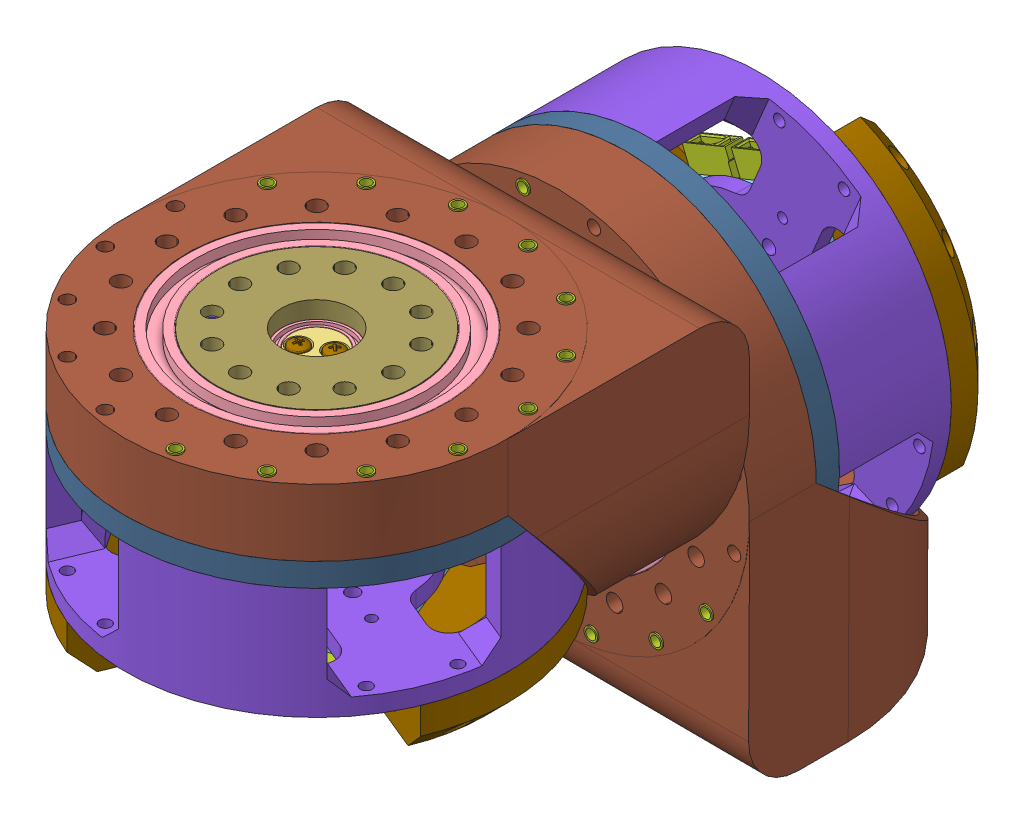
SolidWorks assembly hip, configuration Default. Lengths in mm. (continued)
Components (placement in the parent): (continued)
- Cycloidal_v3-1: Cycloidal_v3 [Default] at (-2.6595 13.4678 32.6634) size (150.25 88 150.25) (continued)
  - foc-motor-controller.step-1: foc-motor-controller.step [Default] at (47.267 33.7573 89.1587) x (-0.382683 0 -0.92388) z (0 -1 0) size (57.23 50 8.13) (continued)
    - R_0603_1608Metric.step-18: R_0603_1608Metric.step [Default] at (-13.3 -20.3875 1.595) x (0 -1 0) z (0 0 1) size (1.6 0.8 0.45)
    - R_0603_1608Metric.step-19: R_0603_1608Metric.step [Default] at (-15.1 -20.3875 1.595) x (0 -1 0) z (0 0 1) size (1.6 0.8 0.45)
    - C_0603_1608Metric.step-17: C_0603_1608Metric.step [Default] at (15.5 -14.4 1.595) x (0 -1 0) z (0 0 1) size (1.6 0.8 0.8)
    - LED_0603_1608Metric.step-1: LED_0603_1608Metric.step [Default] at (-11.5 -23.3875 1.595) x (0 1 0) z (0 0 1) size (1.6 0.8 1.1)
    - C_0805_2012Metric.step-1: C_0805_2012Metric.step [Default] at (19.95 -17 1.595) size (2 1.25 1.25)
    - D_SMB.step-1: D_SMB.step [Default] at (-16.5 11.208 1.595) x (0 -1 0) z (0 0 1) size (5.3 3.55 2.15)
    - C_1206_3216Metric.step-9: C_1206_3216Metric.step [Default] at (-5.3 11 1.595) x (0 1 0) z (0 0 1) size (3.2 1.6 1.6)
    - XT30PW_2_2_-M.G.B.step-2: XT30PW_2_2_-M.G.B.step [Default] at (-20.5 -6.5 1.595) x (0 -1 0) z (-1 0 0) size (15.5 7.1 12.53)
    - C_1206_3216Metric.step-10: C_1206_3216Metric.step [Default] at (1.7 11 1.595) x (0 1 0) z (0 0 1) size (3.2 1.6 1.6)
    - C_1206_3216Metric.step-11: C_1206_3216Metric.step [Default] at (11 11 1.595) x (0 1 0) z (0 0 1) size (3.2 1.6 1.6)
    - C_0603_1608Metric.step-18: C_0603_1608Metric.step [Default] at (-6.3 3.775 1.595) x (0 -1 0) z (0 0 1) size (1.6 0.8 0.8)
    - C_0603_1608Metric.step-19: C_0603_1608Metric.step [Default] at (16.8686 1.7314 1.595) x (0.707107 0.707107 0) z (0 0 1) size (1.6 0.8 0.8)
    - C_0603_1608Metric.step-20: C_0603_1608Metric.step [Default] at (-15.0105 -11.1 1.595) size (1.6 0.8 0.8)
    - C_1206_3216Metric.step-12: C_1206_3216Metric.step [Default] at (-7.7 11 1.595) x (0 1 0) z (0 0 1) size (3.2 1.6 1.6)
    - C_0603_1608Metric.step-21: C_0603_1608Metric.step [Default] at (-18.2 -15.8 1.595) size (1.6 0.8 0.8)
    - C_0603_1608Metric.step-22: C_0603_1608Metric.step [Default] at (-2.1 -11.3 1.595) x (0 -1 0) z (0 0 1) size (1.6 0.8 0.8)
    - C_0603_1608Metric.step-23: C_0603_1608Metric.step [Default] at (-10.8105 -13.4971 1.595) size (1.6 0.8 0.8)
    - C_1206_3216Metric.step-13: C_1206_3216Metric.step [Default] at (4 11 1.595) x (0 1 0) z (0 0 1) size (3.2 1.6 1.6)
    - R_0603_1608Metric.step-20: R_0603_1608Metric.step [Default] at (16 -17.8 1.595) x (0 1 0) z (0 0 1) size (1.6 0.8 0.45)
    - Texas_S-PVSON-N8.step-1: Texas_S-PVSON-N8.step [Default] at (-14.4105 -13.7 1.595) x (-1 0 0) z (0 0 1) size (3 2.98 0.92)
    - C_1206_3216Metric.step-14: C_1206_3216Metric.step [Default] at (21 -2.9 1.595) x (0.707107 -0.707107 0) z (0 0 1) size (3.2 1.6 1.6)
    - C_0603_1608Metric.step-24: C_0603_1608Metric.step [Default] at (-5.9 -16.6 1.595) x (0 1 0) z (0 0 1) size (1.6 0.8 0.8)
    - C_0603_1608Metric.step-25: C_0603_1608Metric.step [Default] at (-3.1 -14.1 1.595) size (1.6 0.8 0.8)
    - R_0603_1608Metric.step-21: R_0603_1608Metric.step [Default] at (7.2 -7.375 1.595) x (0 -1 0) z (0 0 1) size (1.6 0.8 0.45)
    - C_1206_3216Metric.step-15: C_1206_3216Metric.step [Default] at (-0.7 11 1.595) x (0 1 0) z (0 0 1) size (3.2 1.6 1.6)
    - LQFP-64_10x10mm_P0.5mm.step-1: LQFP-64_10x10mm_P0.5mm.step [Default] at (-7 -4.5 1.595) x (-1 0 0) z (0 0 1) size (12 12 1.5)
    - C_0805_2012Metric.step-2: C_0805_2012Metric.step [Default] at (23.35 -17 1.595) x (-1 0 0) z (0 0 1) size (2 1.25 1.25)
    - C_0603_1608Metric.step-26: C_0603_1608Metric.step [Default] at (10.8 -16.8 1.595) x (0 -1 0) z (0 0 1) size (1.6 0.8 0.8)
    - R_0603_1608Metric.step-22: R_0603_1608Metric.step [Default] at (17.5 -17.8 1.595) x (0 -1 0) z (0 0 1) size (1.6 0.8 0.45)
    - C_1206_3216Metric.step-16: C_1206_3216Metric.step [Default] at (20.3 11 1.595) x (0 1 0) z (0 0 1) size (3.2 1.6 1.6)
    - R_0603_1608Metric.step-23: R_0603_1608Metric.step [Default] at (9.2 -16.8 1.595) x (0 -1 0) z (0 0 1) size (1.6 0.8 0.45)
    - C_1206_3216Metric.step-17: C_1206_3216Metric.step [Default] at (-10 11 1.595) x (0 1 0) z (0 0 1) size (3.2 1.6 1.6)
    - R_0603_1608Metric.step-24: R_0603_1608Metric.step [Default] at (17.8 -15.2 1.595) size (1.6 0.8 0.45)
    - C_1206_3216Metric.step-18: C_1206_3216Metric.step [Default] at (19.9 2.6 1.595) x (-0.707107 0.707107 0) z (0 0 1) size (3.2 1.6 1.6)
    - C_0603_1608Metric.step-27: C_0603_1608Metric.step [Default] at (13.4 -7.375 1.595) x (0 -1 0) z (0 0 1) size (1.6 0.8 0.8)
    - R_0603_1608Metric.step-25: R_0603_1608Metric.step [Default] at (8.7 -7.375 1.595) x (0 -1 0) z (0 0 1) size (1.6 0.8 0.45)
    - PQFN-8-EP_6x5mm_P1.27mm_Generic.step-1: PQFN-8-EP_6x5mm_P1.27mm_Generic.step [Default] at (4.9 14.4 -0.085) x (0 1 0) z (0 0 -1) size (6.15 5.15 1.09)
    - C_0805_2012Metric.step-3: C_0805_2012Metric.step [Default] at (-3 8.9 -0.085) x (0 1 0) z (0 0 -1) size (2 1.25 1.25)
    - C_0603_1608Metric.step-28: C_0603_1608Metric.step [Default] at (1.5 -4.3 -0.085) x (0 1 0) z (0 0 -1) size (1.6 0.8 0.8)
    - R_2512_6332Metric.step-1: R_2512_6332Metric.step [Default] at (2.1 8.6 -0.085) x (-1 0 0) z (0 0 -1) size (6.3 3.2 0.6)
    - C_0805_2012Metric.step-4: C_0805_2012Metric.step [Default] at (18.8 8.9 -0.085) x (0 1 0) z (0 0 -1) size (2 1.25 1.25)
    - C_0805_2012Metric.step-5: C_0805_2012Metric.step [Default] at (-5.2 8.901 -0.085) x (0 1 0) z (0 0 -1) size (2 1.25 1.25)
    - PQFN-8-EP_6x5mm_P1.27mm_Generic.step-2: PQFN-8-EP_6x5mm_P1.27mm_Generic.step [Default] at (16.9 14.6 -0.085) x (0 -1 0) z (0 0 -1) size (6.15 5.15 1.09)
    - PQFN-8-EP_6x5mm_P1.27mm_Generic.step-3: PQFN-8-EP_6x5mm_P1.27mm_Generic.step [Default] at (-1.1 14.6 -0.085) x (0 -1 0) z (0 0 -1) size (6.15 5.15 1.09)
    - R_0603_1608Metric.step-26: R_0603_1608Metric.step [Default] at (8.2 8.8 -0.085) x (0 1 0) z (0 0 -1) size (1.6 0.8 0.45)
    - R_2512_6332Metric.step-2: R_2512_6332Metric.step [Default] at (-10.3 8.601 -0.085) x (1 0 0) z (0 0 -1) size (6.3 3.2 0.6)
    - TSSOP-16_4.4x5mm_P0.65mm.step-1: TSSOP-16_4.4x5mm_P0.65mm.step [Default] at (0 0 -0.085) x (-1 0 0) z (0 0 -1) size (6.4 5 1.1)
    - C_0603_1608Metric.step-29: C_0603_1608Metric.step [Default] at (0 -4.25 -0.085) x (0 1 0) z (0 0 -1) size (1.6 0.8 0.8)
    - PQFN-8-EP_6x5mm_P1.27mm_Generic.step-4: PQFN-8-EP_6x5mm_P1.27mm_Generic.step [Default] at (10.9 14.4 -0.085) x (0 1 0) z (0 0 -1) size (6.15 5.15 1.09)
    - R_2512_6332Metric.step-3: R_2512_6332Metric.step [Default] at (13.7 8.6 -0.085) x (1 0 0) z (0 0 -1) size (6.3 3.2 0.6)
    - PQFN-8-EP_6x5mm_P1.27mm_Generic.step-5: PQFN-8-EP_6x5mm_P1.27mm_Generic.step [Default] at (-13.1 14.401 -0.085) x (0 1 0) z (0 0 -1) size (6.15 5.15 1.09)
    - C_0603_1608Metric.step-30: C_0603_1608Metric.step [Default] at (-1.5 -4.3 -0.085) x (0 -1 0) z (0 0 -1) size (1.6 0.8 0.8)
    - PQFN-8-EP_6x5mm_P1.27mm_Generic.step-6: PQFN-8-EP_6x5mm_P1.27mm_Generic.step [Default] at (-7.1 14.601 -0.085) x (0 -1 0) z (0 0 -1) size (6.15 5.15 1.09)
    - foc-motor-controller_PCB.step-1: foc-motor-controller_PCB.step [Default] at origin size (50 50 1.51)
  - hex nut style 1 gradeab_iso-1: hex nut style 1 gradeab_iso [ISO - 4032 - M3 - W - N] at (35.6313 33.7573 117.2498) x (1 0 0) z (0 -1 0) size (5.5 6.35 2.4)
  - Cycloidal_Discs_8308-1: Cycloidal_Discs_8308 [Default] at (6.9481 42.227 30.6143) x (0.999764 0 -0.021738) z (0.021738 0 0.999764) size (79.25 5 79.73)
    - Cycloidal_Discs-1: Cycloidal_Discs [Default] at (38.3081 39.5303 58.0959) size (79.25 5 79.73)
    - radial ball bearing_68_iso-1: radial ball bearing_68_iso [ISO 15 RBB - 274 - 14,SI,NC,14_68] at (18.3896 43.2803 46.5959) x (0 1 0) z (0 0 1) size (2.5 7 7)
    - radial ball bearing_68_iso-2: radial ball bearing_68_iso [ISO 15 RBB - 274 - 14,SI,NC,14_68] at (38.3081 43.2803 81.0959) x (0 1 0) z (0 0 1) size (2.5 7 7)
    - radial ball bearing_68_iso-3: radial ball bearing_68_iso [ISO 15 RBB - 274 - 14,SI,NC,14_68] at (18.3896 43.2803 69.5959) x (0 1 0) z (0 0 1) size (2.5 7 7)
    - radial ball bearing_68_iso-4: radial ball bearing_68_iso [ISO 15 RBB - 274 - 14,SI,NC,14_68] at (38.3081 43.2803 35.0959) x (0 1 0) z (0 0 1) size (2.5 7 7)
    - radial ball bearing_68_iso-5: radial ball bearing_68_iso [ISO 15 RBB - 274 - 14,SI,NC,14_68] at (58.2267 43.2803 69.5959) x (0 1 0) z (0 0 1) size (2.5 7 7)
    - radial ball bearing_68_iso-6: radial ball bearing_68_iso [ISO 15 RBB - 274 - 14,SI,NC,14_68] at (58.2267 43.2803 46.5959) x (0 1 0) z (0 0 1) size (2.5 7 7)
  - Cycloidal_Discs_8308-2: Cycloidal_Discs_8308 [Default] at (85.7348 37.227 31.9683) x (0.403317 0 0.91506) z (-0.91506 0 0.403317) size (79.25 5 79.73)
    - Cycloidal_Discs-1: Cycloidal_Discs [Default] at (38.3081 39.5303 58.0959) size (79.25 5 79.73)
    - radial ball bearing_68_iso-1: radial ball bearing_68_iso [ISO 15 RBB - 274 - 14,SI,NC,14_68] at (18.3896 43.2803 46.5959) x (0 1 0) z (0 0 1) size (2.5 7 7)
    - radial ball bearing_68_iso-2: radial ball bearing_68_iso [ISO 15 RBB - 274 - 14,SI,NC,14_68] at (38.3081 43.2803 81.0959) x (0 1 0) z (0 0 1) size (2.5 7 7)
    - radial ball bearing_68_iso-3: radial ball bearing_68_iso [ISO 15 RBB - 274 - 14,SI,NC,14_68] at (18.3896 43.2803 69.5959) x (0 1 0) z (0 0 1) size (2.5 7 7)
    - radial ball bearing_68_iso-4: radial ball bearing_68_iso [ISO 15 RBB - 274 - 14,SI,NC,14_68] at (38.3081 43.2803 35.0959) x (0 1 0) z (0 0 1) size (2.5 7 7)
    - radial ball bearing_68_iso-5: radial ball bearing_68_iso [ISO 15 RBB - 274 - 14,SI,NC,14_68] at (58.2267 43.2803 69.5959) x (0 1 0) z (0 0 1) size (2.5 7 7)
    - radial ball bearing_68_iso-6: radial ball bearing_68_iso [ISO 15 RBB - 274 - 14,SI,NC,14_68] at (58.2267 43.2803 46.5959) x (0 1 0) z (0 0 1) size (2.5 7 7)
  - m6-1: m6 [Default] at (27.3484 93.9895 100.6587) x (-0.80367 0 -0.595076) z (-0.595076 0 0.80367) size (6 16 6)
  - Motor_Cover_v2-2: Motor_Cover_v2 [Default] at (47.267 36.1573 89.1587) x (-0.92388 0 -0.382683) z (0.382683 0 -0.92388) size (115 33.6 115)
  - driver_cover-1: driver_cover [Default] at (47.267 36.1573 89.1587) x (-0.384295 0 -0.92321) z (-0.92321 0 0.384295) size (81.32 15 115)
  - Base_plate_2-1: Base_plate_2 [Default] at (47.267 69.7573 89.1587) size (115 7 115)
  - Cover_new-1: Cover_new [Default] at (47.267 86.8173 89.1587) size (115 87.56 130)
  - Output_Shaft-1: Output_Shaft [Default] at (47.267 86.8173 89.1587) size (60 10 60)
- Cycloidal_v3-2: Cycloidal_v3 [Default] at (91.3873 -36.6902 -47.4953) x (-0.999985 0.005457 0) z (0.005457 0.999985 0) size (150.25 88 150.25)
  - motor-X83008S.stp-1: motor-X83008S.stp [Default] at (85.5027 89.8915 67.8666) x (-0.706334 0 0.707879) z (0 -1 0) size (114.7 114.7 37.62) (hidden)
    - base.stp-1: base.stp [Default] at (42.0794 12.0269 46.7342) size (91.6 91.6 15.61)
    - stator.stp-1: stator.stp [Default] at (42.0794 12.0269 33.1342) x (0.08493 -0.996387 0) z (0 0 1) size (83 83 8)
    - coil.stp-1: coil.stp [Default] at (39.5332 41.8984 37.1342) x (0.996387 0.08493 0) z (-0.08493 0.996387 0) size (4.4 10.2 10.5)
    - coil.stp-2: coil.stp [Default] at (34.3848 41.0025 37.1342) x (0.966502 0.256661 0) z (-0.256661 0.966502 0) size (4.4 10.2 10.5)
    - coil.stp-3: coil.stp [Default] at (29.4701 39.2261 37.1342) x (0.90725 0.420593 0) z (-0.420593 0.90725 0) size (4.4 10.2 10.5)
    - coil.stp-4: coil.stp [Default] at (24.9386 36.6233 37.1342) x (0.820431 0.571745 0) z (-0.571745 0.820431 0) size (4.4 10.2 10.5)
    - coil.stp-5: coil.stp [Default] at (20.9279 33.2732 37.1342) x (0.708685 0.705525 0) z (-0.705525 0.708685 0) size (4.4 10.2 10.5)
    - coil.stp-6: coil.stp [Default] at (17.5599 29.2775 37.1342) x (0.575405 0.817869 0) z (-0.817869 0.575405 0) size (4.4 10.2 10.5)
    - coil.stp-7: coil.stp [Default] at (14.9368 24.7576 37.1342) x (0.424642 0.905361 0) z (-0.905361 0.424642 0) size (4.4 10.2 10.5)
    - coil.stp-8: coil.stp [Default] at (13.1385 19.8509 37.1342) x (0.260976 0.965345 0) z (-0.965345 0.260976 0) size (4.4 10.2 10.5)
    - coil.stp-9: coil.stp [Default] at (12.2196 14.7066 37.1342) x (0.089381 0.995998 0) z (-0.995998 0.089381 0) size (4.4 10.2 10.5)
    - coil.stp-10: coil.stp [Default] at (12.2079 9.4807 37.1342) x (-0.08493 0.996387 0) z (-0.996387 -0.08493 0) size (4.4 10.2 10.5)
    - coil.stp-11: coil.stp [Default] at (13.1039 4.3323 37.1342) x (-0.256661 0.966502 0) z (-0.966502 -0.256661 0) size (4.4 10.2 10.5)
    - coil.stp-12: coil.stp [Default] at (14.8802 -0.5824 37.1342) x (-0.420593 0.90725 0) z (-0.90725 -0.420593 0) size (4.4 10.2 10.5)
    - coil.stp-13: coil.stp [Default] at (17.483 -5.1139 37.1342) x (-0.571745 0.820431 0) z (-0.820431 -0.571745 0) size (4.4 10.2 10.5)
    - coil.stp-14: coil.stp [Default] at (20.8332 -9.1246 37.1342) x (-0.705525 0.708685 0) z (-0.708685 -0.705525 0) size (4.4 10.2 10.5)
    - coil.stp-15: coil.stp [Default] at (24.8289 -12.4926 37.1342) x (-0.817869 0.575405 0) z (-0.575405 -0.817869 0) size (4.4 10.2 10.5)
    - coil.stp-16: coil.stp [Default] at (29.3487 -15.1157 37.1342) x (-0.905361 0.424642 0) z (-0.424642 -0.905361 0) size (4.4 10.2 10.5)
    - coil.stp-17: coil.stp [Default] at (34.2554 -16.914 37.1342) x (-0.965345 0.260976 0) z (-0.260976 -0.965345 0) size (4.4 10.2 10.5)
    - coil.stp-18: coil.stp [Default] at (39.3998 -17.8329 37.1342) x (-0.995998 0.089381 0) z (-0.089381 -0.995998 0) size (4.4 10.2 10.5)
    - coil.stp-19: coil.stp [Default] at (44.6256 -17.8446 37.1342) x (-0.996387 -0.08493 0) z (0.08493 -0.996387 0) size (4.4 10.2 10.5)
    - coil.stp-20: coil.stp [Default] at (49.7741 -16.9486 37.1342) x (-0.966502 -0.256661 0) z (0.256661 -0.966502 0) size (4.4 10.2 10.5)
    - coil.stp-21: coil.stp [Default] at (54.6887 -15.1723 37.1342) x (-0.90725 -0.420593 0) z (0.420593 -0.90725 0) size (4.4 10.2 10.5)
    - coil.stp-22: coil.stp [Default] at (59.2202 -12.5695 37.1342) x (-0.820431 -0.571745 0) z (0.571745 -0.820431 0) size (4.4 10.2 10.5)
    - coil.stp-23: coil.stp [Default] at (63.2309 -9.2193 37.1342) x (-0.708685 -0.705525 0) z (0.705525 -0.708685 0) size (4.4 10.2 10.5)
    - coil.stp-24: coil.stp [Default] at (66.599 -5.2236 37.1342) x (-0.575405 -0.817869 0) z (0.817869 -0.575405 0) size (4.4 10.2 10.5)
    - coil.stp-25: coil.stp [Default] at (69.222 -0.7038 37.1342) x (-0.424642 -0.905361 0) z (0.905361 -0.424642 0) size (4.4 10.2 10.5)
    - coil.stp-26: coil.stp [Default] at (71.0203 4.2029 37.1342) x (-0.260976 -0.965345 0) z (0.965345 -0.260976 0) size (4.4 10.2 10.5)
    - coil.stp-27: coil.stp [Default] at (71.9392 9.3473 37.1342) x (-0.089381 -0.995998 0) z (0.995998 -0.089381 0) size (4.4 10.2 10.5)
    - coil.stp-28: coil.stp [Default] at (71.9509 14.5731 37.1342) x (0.08493 -0.996387 0) z (0.996387 0.08493 0) size (4.4 10.2 10.5)
    - coil.stp-29: coil.stp [Default] at (71.055 19.7216 37.1342) x (0.256661 -0.966502 0) z (0.966502 0.256661 0) size (4.4 10.2 10.5)
    - coil.stp-30: coil.stp [Default] at (69.2786 24.6362 37.1342) x (0.420593 -0.90725 0) z (0.90725 0.420593 0) size (4.4 10.2 10.5)
    - coil.stp-31: coil.stp [Default] at (66.6758 29.1677 37.1342) x (0.571745 -0.820431 0) z (0.820431 0.571745 0) size (4.4 10.2 10.5)
    - coil.stp-32: coil.stp [Default] at (63.3257 33.1785 37.1342) x (0.705525 -0.708685 0) z (0.708685 0.705525 0) size (4.4 10.2 10.5)
    - coil.stp-33: coil.stp [Default] at (59.33 36.5465 37.1342) x (0.817869 -0.575405 0) z (0.575405 0.817869 0) size (4.4 10.2 10.5)
    - coil.stp-34: coil.stp [Default] at (54.8101 39.1695 37.1342) x (0.905361 -0.424642 0) z (0.424642 0.905361 0) size (4.4 10.2 10.5)
    - coil.stp-35: coil.stp [Default] at (49.9034 40.9678 37.1342) x (0.965345 -0.260976 0) z (0.260976 0.965345 0) size (4.4 10.2 10.5)
    - coil.stp-36: coil.stp [Default] at (44.759 41.8868 37.1342) x (0.995998 -0.089381 0) z (0.089381 0.995998 0) size (4.4 10.2 10.5)
    - rotor.stp-1: rotor.stp [Default] at (42.0794 12.0269 42.1342) x (-0.293442 0.955977 0) z (0 0 -1) size (91.8 91.8 12)
    - outrunner.stp-1: outrunner.stp [Default] at (42.0794 12.0269 30.1342) x (-0.254711 0.967017 0) z (-0.967017 -0.254711 0) size (91.8 17.01 91.8)
    - screw-mount.stp-1: screw-mount.stp [Default] at (38.1314 27.0157 27.1342) x (1 0 0) z (0 0 -1) size (7 7 6.5)
    - screw-mount.stp-2: screw-mount.stp [Default] at (27.0906 8.0789 27.1342) x (1 0 0) z (0 0 -1) size (7 7 6.5)
    - screw-mount.stp-3: screw-mount.stp [Default] at (57.0682 15.9749 27.1342) x (1 0 0) z (0 0 -1) size (7 7 6.5)
    - screw-mount.stp-4: screw-mount.stp [Default] at (46.0274 -2.9618 27.1342) x (1 0 0) z (0 0 -1) size (7 7 6.5)
    - 6702ZZ-bearing-15x21x4.stp-1: 6702ZZ-bearing-15x21x4.stp [Default] at (42.0794 12.0269 43.7342) x (1 0 0) z (0 -1 0) size (21 4 21)
    - 6702ZZ-bearing-15x21x4.stp-2: 6702ZZ-bearing-15x21x4.stp [Default] at (42.0794 12.0269 35.1342) x (1 0 0) z (0 1 0) size (21 4 21)
    - shaft.stp-1: shaft.stp [Default] at (42.0794 12.0269 20.1342) size (16 16 31.6)
    - fix-screw.stp-1: fix-screw.stp [Default] at (42.0794 12.0269 51.7342) x (1 0 0) z (0 0 -1) size (19.67 18.96 12.02)
  - Base_Plate-1: Base_Plate [Default] at (47.267 69.7573 89.1587) x (0.863342 0 -0.50462) z (0.50462 0 0.863342) size (40 7 40)
  - Eccentric_Shaft-1: Eccentric_Shaft [Default] at (38.9525 70.4165 102.8564) x (-0.50462 0 -0.863342) z (0.863342 0 -0.50462) size (20 15 17)
    - Eccentric_Shaft_bot-1: Eccentric_Shaft_bot [Default] at (7.6302 6.3409 14.0904) size (17 5 17)
    - Eccentric_Shaft_bot-2: Eccentric_Shaft_bot [Default] at (7.6302 11.3409 14.0904) x (-1 0 0) z (0 0 -1) size (17 5 17)
    - Eccentric_Shaft_top-1: Eccentric_Shaft_top [Default] at (7.6302 16.3409 14.0904) x (-1 0 0) z (0 0 -1) size (17 5 17)
  - radial ball bearing_68_iso-39: radial ball bearing_68_iso [ISO 15 RBB - 1860 - 32,SI,NC,32_68] at (47.267 91.8173 89.1587) x (0 1 0) z (0.105786 0 0.994389) size (10 78 78)
  - radial ball bearing_68_iso-40: radial ball bearing_68_iso [ISO 15 RBB - 1840 - 32,SI,NC,32_68] at (47.267 73.2573 89.1587) x (0 1 0) z (-0.019534 0 0.999809) size (7 52 52)
  - m13_bearing-31: m13_bearing [Default] at (-10.7414 95.4081 67.0593) x (0.227678 0 0.973736) z (0.973736 0 -0.227678) size (13 16 13)
    - m6-1: m6 [Default] at (8.4921 2.5508 14.8914) size (6 16 6)
    - radial ball bearing_68_iso-1: radial ball bearing_68_iso [ISO 15 RBB - 286 - 10,SI,NC,10_68] at (8.4921 16.0508 14.8914) x (0 1 0) z (0 0 1) size (5 13 13)
    - radial ball bearing_68_iso-2: radial ball bearing_68_iso [ISO 15 RBB - 286 - 10,SI,NC,10_68] at (8.4921 11.0508 14.8914) x (0 1 0) z (0 0 1) size (5 13 13)
  - m13_bearing-32: m13_bearing [Default] at (-14.1668 95.4081 84.2801) x (0.227678 0 0.973736) z (0.973736 0 -0.227678) size (13 16 13)
    - m6-1: m6 [Default] at (8.4921 2.5508 14.8914) size (6 16 6)
    - radial ball bearing_68_iso-1: radial ball bearing_68_iso [ISO 15 RBB - 286 - 10,SI,NC,10_68] at (8.4921 16.0508 14.8914) x (0 1 0) z (0 0 1) size (5 13 13)
    - radial ball bearing_68_iso-2: radial ball bearing_68_iso [ISO 15 RBB - 286 - 10,SI,NC,10_68] at (8.4921 11.0508 14.8914) x (0 1 0) z (0 0 1) size (5 13 13)
  - m13_bearing-34: m13_bearing [Default] at (13.6125 95.5581 125.8547) x (0.227678 0 0.973736) z (0.973736 0 -0.227678) size (13 16 13)
    - m6-1: m6 [Default] at (8.4921 2.5508 14.8914) size (6 16 6)
    - radial ball bearing_68_iso-1: radial ball bearing_68_iso [ISO 15 RBB - 286 - 10,SI,NC,10_68] at (8.4921 16.0508 14.8914) x (0 1 0) z (0 0 1) size (5 13 13)
    - radial ball bearing_68_iso-2: radial ball bearing_68_iso [ISO 15 RBB - 286 - 10,SI,NC,10_68] at (8.4921 11.0508 14.8914) x (0 1 0) z (0 0 1) size (5 13 13)
  - m13_bearing-35: m13_bearing [Default] at (-0.9866 95.4081 116.0999) x (0.227678 0 0.973736) z (0.973736 0 -0.227678) size (13 16 13)
    - m6-1: m6 [Default] at (8.4921 2.5508 14.8914) size (6 16 6)
    - radial ball bearing_68_iso-1: radial ball bearing_68_iso [ISO 15 RBB - 286 - 10,SI,NC,10_68] at (8.4921 16.0508 14.8914) x (0 1 0) z (0 0 1) size (5 13 13)
    - radial ball bearing_68_iso-2: radial ball bearing_68_iso [ISO 15 RBB - 286 - 10,SI,NC,10_68] at (8.4921 11.0508 14.8914) x (0 1 0) z (0 0 1) size (5 13 13)
  - m13_bearing-36: m13_bearing [Default] at (-10.7414 95.5581 101.5009) x (0.227678 0 0.973736) z (0.973736 0 -0.227678) size (13 16 13)
    - m6-1: m6 [Default] at (8.4921 2.5508 14.8914) size (6 16 6)
    - radial ball bearing_68_iso-1: radial ball bearing_68_iso [ISO 15 RBB - 286 - 10,SI,NC,10_68] at (8.4921 16.0508 14.8914) x (0 1 0) z (0 0 1) size (5 13 13)
    - radial ball bearing_68_iso-2: radial ball bearing_68_iso [ISO 15 RBB - 286 - 10,SI,NC,10_68] at (8.4921 11.0508 14.8914) x (0 1 0) z (0 0 1) size (5 13 13)
  - m13_bearing-1: m13_bearing [Default] at (-0.8801 95.4081 62.5627) x (0.736525 0 0.676411) z (0.676411 0 -0.736525) size (13 16 13)
    - m6-1: m6 [Default] at (8.4921 2.5508 14.8914) size (6 16 6)
    - radial ball bearing_68_iso-1: radial ball bearing_68_iso [ISO 15 RBB - 286 - 10,SI,NC,10_68] at (8.4921 16.0508 14.8914) x (0 1 0) z (0 0 1) size (5 13 13)
    - radial ball bearing_68_iso-2: radial ball bearing_68_iso [ISO 15 RBB - 286 - 10,SI,NC,10_68] at (8.4921 11.0508 14.8914) x (0 1 0) z (0 0 1) size (5 13 13)
  - m13_bearing-2: m13_bearing [Default] at (48.6831 95.4081 124.0939) x (0.120271 0 0.992741) z (0.992741 0 -0.120271) size (13 16 13)
    - m6-1: m6 [Default] at (8.4921 2.5508 14.8914) size (6 16 6)
    - radial ball bearing_68_iso-1: radial ball bearing_68_iso [ISO 15 RBB - 286 - 10,SI,NC,10_68] at (8.4921 16.0508 14.8914) x (0 1 0) z (0 0 1) size (5 13 13)
    - radial ball bearing_68_iso-2: radial ball bearing_68_iso [ISO 15 RBB - 286 - 10,SI,NC,10_68] at (8.4921 11.0508 14.8914) x (0 1 0) z (0 0 1) size (5 13 13)
  - m13_bearing-3: m13_bearing [Default] at (32.7832 95.4081 34.9886) x (-0.046141 0 0.998935) z (0.998935 0 0.046141) size (13 16 13)
    - m6-1: m6 [Default] at (8.4921 2.5508 14.8914) size (6 16 6)
    - radial ball bearing_68_iso-1: radial ball bearing_68_iso [ISO 15 RBB - 286 - 10,SI,NC,10_68] at (8.4921 16.0508 14.8914) x (0 1 0) z (0 0 1) size (5 13 13)
    - radial ball bearing_68_iso-2: radial ball bearing_68_iso [ISO 15 RBB - 286 - 10,SI,NC,10_68] at (8.4921 11.0508 14.8914) x (0 1 0) z (0 0 1) size (5 13 13)
  - m13_bearing-4: m13_bearing [Default] at (77.6928 95.3081 80.133) x (-0.036208 0 0.999344) z (0.999344 0 0.036208) size (13 16 13)
    - m6-1: m6 [Default] at (8.4921 2.5508 14.8914) size (6 16 6)
    - radial ball bearing_68_iso-1: radial ball bearing_68_iso [ISO 15 RBB - 286 - 10,SI,NC,10_68] at (8.4921 16.0508 14.8914) x (0 1 0) z (0 0 1) size (5 13 13)
    - radial ball bearing_68_iso-2: radial ball bearing_68_iso [ISO 15 RBB - 286 - 10,SI,NC,10_68] at (8.4921 11.0508 14.8914) x (0 1 0) z (0 0 1) size (5 13 13)
  - m13_bearing-5: m13_bearing [Default] at (73.474 95.4081 98.7828) x (0.059133 0 0.99825) z (0.99825 0 -0.059133) size (13 16 13)
    - m6-1: m6 [Default] at (8.4921 2.5508 14.8914) size (6 16 6)
    - radial ball bearing_68_iso-1: radial ball bearing_68_iso [ISO 15 RBB - 286 - 10,SI,NC,10_68] at (8.4921 16.0508 14.8914) x (0 1 0) z (0 0 1) size (5 13 13)
    - radial ball bearing_68_iso-2: radial ball bearing_68_iso [ISO 15 RBB - 286 - 10,SI,NC,10_68] at (8.4921 11.0508 14.8914) x (0 1 0) z (0 0 1) size (5 13 13)
  - m13_bearing-6: m13_bearing [Default] at (12.9248 95.4081 46.7315) x (0.451561 0 0.89224) z (0.89224 0 -0.451561) size (13 16 13)
    - m6-1: m6 [Default] at (8.4921 2.5508 14.8914) size (6 16 6)
    - radial ball bearing_68_iso-1: radial ball bearing_68_iso [ISO 15 RBB - 286 - 10,SI,NC,10_68] at (8.4921 16.0508 14.8914) x (0 1 0) z (0 0 1) size (5 13 13)
    - radial ball bearing_68_iso-2: radial ball bearing_68_iso [ISO 15 RBB - 286 - 10,SI,NC,10_68] at (8.4921 11.0508 14.8914) x (0 1 0) z (0 0 1) size (5 13 13)
  - m13_bearing-7: m13_bearing [Default] at (56.6452 95.4081 32.3406) x (-0.545813 0 0.837907) z (0.837907 0 0.545813) size (13 16 13)
    - m6-1: m6 [Default] at (8.4921 2.5508 14.8914) size (6 16 6)
    - radial ball bearing_68_iso-1: radial ball bearing_68_iso [ISO 15 RBB - 286 - 10,SI,NC,10_68] at (8.4921 16.0508 14.8914) x (0 1 0) z (0 0 1) size (5 13 13)
    - radial ball bearing_68_iso-2: radial ball bearing_68_iso [ISO 15 RBB - 286 - 10,SI,NC,10_68] at (8.4921 11.0508 14.8914) x (0 1 0) z (0 0 1) size (5 13 13)
  - m13_bearing-8: m13_bearing [Default] at (63.0373 95.4081 51.3153) x (0.158553 0 0.98735) z (0.98735 0 -0.158553) size (13 16 13)
    - m6-1: m6 [Default] at (8.4921 2.5508 14.8914) size (6 16 6)
    - radial ball bearing_68_iso-1: radial ball bearing_68_iso [ISO 15 RBB - 286 - 10,SI,NC,10_68] at (8.4921 16.0508 14.8914) x (0 1 0) z (0 0 1) size (5 13 13)
    - radial ball bearing_68_iso-2: radial ball bearing_68_iso [ISO 15 RBB - 286 - 10,SI,NC,10_68] at (8.4921 11.0508 14.8914) x (0 1 0) z (0 0 1) size (5 13 13)
  - m13_bearing-9: m13_bearing [Default] at (83.8577 95.4081 55.5358) x (-0.687134 0 0.72653) z (0.72653 0 0.687134) size (13 16 13)
    - m6-1: m6 [Default] at (8.4921 2.5508 14.8914) size (6 16 6)
    - radial ball bearing_68_iso-1: radial ball bearing_68_iso [ISO 15 RBB - 286 - 10,SI,NC,10_68] at (8.4921 16.0508 14.8914) x (0 1 0) z (0 0 1) size (5 13 13)
    - radial ball bearing_68_iso-2: radial ball bearing_68_iso [ISO 15 RBB - 286 - 10,SI,NC,10_68] at (8.4921 11.0508 14.8914) x (0 1 0) z (0 0 1) size (5 13 13)
  - m13_bearing-11: m13_bearing [Default] at (30.1977 95.4081 135.7424) x (0.57351 0 0.819198) z (0.819198 0 -0.57351) size (13 16 13)
    - m6-1: m6 [Default] at (8.4921 2.5508 14.8914) size (6 16 6)
    - radial ball bearing_68_iso-1: radial ball bearing_68_iso [ISO 15 RBB - 286 - 10,SI,NC,10_68] at (8.4921 16.0508 14.8914) x (0 1 0) z (0 0 1) size (5 13 13)
    - radial ball bearing_68_iso-2: radial ball bearing_68_iso [ISO 15 RBB - 286 - 10,SI,NC,10_68] at (8.4921 11.0508 14.8914) x (0 1 0) z (0 0 1) size (5 13 13)
  - m13_bearing-12: m13_bearing [Default] at (62.8861 95.4081 115.3744) x (0.184178 0 0.982893) z (0.982893 0 -0.184178) size (13 16 13)
    - m6-1: m6 [Default] at (8.4921 2.5508 14.8914) size (6 16 6)
    - radial ball bearing_68_iso-1: radial ball bearing_68_iso [ISO 15 RBB - 286 - 10,SI,NC,10_68] at (8.4921 16.0508 14.8914) x (0 1 0) z (0 0 1) size (5 13 13)
    - radial ball bearing_68_iso-2: radial ball bearing_68_iso [ISO 15 RBB - 286 - 10,SI,NC,10_68] at (8.4921 11.0508 14.8914) x (0 1 0) z (0 0 1) size (5 13 13)
  - socket button head screw_iso-2: socket button head screw_iso [ISO 7380 - M4 x 12 - 12N] at (47.267 67.4573 134.1587) x (0 1 0) z (-0.724148 0 0.689645) size (14.2 7.6 7.6)
  - socket button head screw_iso-3: socket button head screw_iso [ISO 7380 - M4 x 12 - 12N] at (15.4472 67.4573 57.3389) x (0 1 0) z (-0.724148 0 0.689645) size (14.2 7.6 7.6)
  - socket button head screw_iso-4: socket button head screw_iso [ISO 7380 - M4 x 12 - 12N] at (30.0462 67.4573 47.5841) x (0 1 0) z (-0.724148 0 0.689645) size (14.2 7.6 7.6)
  - socket button head screw_iso-5: socket button head screw_iso [ISO 7380 - M4 x 12 - 12N] at (47.267 67.4573 44.1587) x (0 1 0) z (-0.724148 0 0.689645) size (14.2 7.6 7.6)
  - socket button head screw_iso-6: socket button head screw_iso [ISO 7380 - M4 x 12 - 12N] at (64.4877 67.4573 47.5841) x (0 1 0) z (-0.724148 0 0.689645) size (14.2 7.6 7.6)
  - socket button head screw_iso-8: socket button head screw_iso [ISO 7380 - M4 x 12 - 12N] at (88.8416 67.4573 71.9379) x (0 1 0) z (-0.724148 0 0.689645) size (14.2 7.6 7.6)
  - socket button head screw_iso-9: socket button head screw_iso [ISO 7380 - M4 x 12 - 12N] at (92.267 67.4573 89.1587) x (0 1 0) z (-0.724148 0 0.689645) size (14.2 7.6 7.6)
  - socket button head screw_iso-10: socket button head screw_iso [ISO 7380 - M4 x 12 - 12N] at (88.8416 67.4573 106.3794) x (0 1 0) z (-0.724148 0 0.689645) size (14.2 7.6 7.6)
  - socket button head screw_iso-11: socket button head screw_iso [ISO 7380 - M4 x 12 - 12N] at (79.0868 67.4573 120.9785) x (0 1 0) z (-0.724148 0 0.689645) size (14.2 7.6 7.6)
  - M3x4x4.2_brass_insert-2: M3x4x4.2_brass_insert [Default] at (2.3676 97.2573 59.1579) x (-0.680278 0 -0.732954) z (-0.732954 0 0.680278) size (4 4 4)
  - M3x4x4.2_brass_insert-3: M3x4x4.2_brass_insert [Default] at (17.2662 97.2573 44.2593) x (-0.509546 0 -0.860444) z (-0.860444 0 0.509546) size (4 4 4)
  - M3x4x4.2_brass_insert-6: M3x4x4.2_brass_insert [Default] at (77.2678 97.2573 44.2593) x (-0.680278 0 -0.732954) z (-0.732954 0 0.680278) size (4 4 4)
  - M3x4x4.2_brass_insert-8: M3x4x4.2_brass_insert [Default] at (100.2294 93.2573 78.6238) x (-0.970393 0 0.241533) z (-0.241533 0 -0.970393) size (4 4 4)
  - M3x4x4.2_brass_insert-14: M3x4x4.2_brass_insert [Default] at (36.7321 97.2573 36.1963) x (0.509546 0 0.860444) z (0.860444 0 -0.509546) size (4 4 4)
  - M3x4x4.2_brass_insert-15: M3x4x4.2_brass_insert [Default] at (57.8019 93.2573 36.1963) x (0.897191 0 -0.441644) z (0.441644 0 0.897191) size (4 4 4)
  - M3x4x4.2_brass_insert-16: M3x4x4.2_brass_insert [Default] at (92.1663 97.2573 59.1579) x (-0.680278 0 -0.732954) z (-0.732954 0 0.680278) size (4 4 4)
  - M3x4x4.2_brass_insert-17: M3x4x4.2_brass_insert [Default] at (100.2294 97.2573 99.6935) x (0.680278 0 0.732954) z (0.732954 0 -0.680278) size (4 4 4)
  - M3x4x4.2_brass_insert-19: M3x4x4.2_brass_insert [Default] at (92.1663 97.2573 119.1595) x (0.680278 0 0.732954) z (0.732954 0 -0.680278) size (4 4 4)
  - M3x4x4.2_brass_insert-20: M3x4x4.2_brass_insert [Default] at (77.2678 97.2573 134.058) x (0.680278 0 0.732954) z (0.732954 0 -0.680278) size (4 4 4)
  - M3x4x4.2_brass_insert-21: M3x4x4.2_brass_insert [Default] at (57.8019 97.2573 142.1211) x (0.680278 0 0.732954) z (0.732954 0 -0.680278) size (4 4 4)
  - M4x6x5.5_brass_insert-47: M4x6x5.5_brass_insert [Default] at (5.6924 92.8573 71.9379) x (0.474598 0 0.880203) z (0 1 0) size (5 5 6)
  - M4x6x5.5_brass_insert-48: M4x6x5.5_brass_insert [Default] at (2.267 92.8573 89.1587) x (0.260051 0 0.965595) z (0 1 0) size (5 5 6)
  - M4x6x5.5_brass_insert-49: M4x6x5.5_brass_insert [Default] at (5.6924 87.0073 106.3794) x (-0.745833 0 0.666133) z (0 -1 0) size (5 5 6)
  - M4x6x5.5_brass_insert-50: M4x6x5.5_brass_insert [Default] at (15.4472 86.8573 120.9785) x (-0.745833 0 0.666133) z (0 -1 0) size (5 5 6)
  - M4x6x5.5_brass_insert-51: M4x6x5.5_brass_insert [Default] at (30.0462 87.0073 130.7332) x (0.260051 0 -0.965595) z (0 -1 0) size (5 5 6)
  - M4x6x5.5_brass_insert-6: M4x6x5.5_brass_insert [Default] at (27.3484 93.9895 100.6587) x (0.252509 0 0.967595) z (0 1 0) size (5 5 6)
  - M4x6x5.5_brass_insert-20: M4x6x5.5_brass_insert [Default] at (64.4877 86.8573 130.7332) x (-0.745833 0 0.666133) z (0 -1 0) size (5 5 6)
  - M4x6x5.5_brass_insert-21: M4x6x5.5_brass_insert [Default] at (47.267 86.8573 134.1587) x (-0.745833 0 0.666133) z (0 -1 0) size (5 5 6)
  - M4x6x5.5_brass_insert-22: M4x6x5.5_brass_insert [Default] at (15.4472 86.8573 57.3389) x (0.623293 0 0.781988) z (0 -1 0) size (5 5 6)
  - M4x6x5.5_brass_insert-23: M4x6x5.5_brass_insert [Default] at (30.0462 86.8573 47.5841) x (0.623293 0 0.781988) z (0 -1 0) size (5 5 6)
  - M4x6x5.5_brass_insert-24: M4x6x5.5_brass_insert [Default] at (79.0868 86.8573 120.9785) x (0.541965 0 0.840401) z (0 -1 0) size (5 5 6)
  - M4x6x5.5_brass_insert-25: M4x6x5.5_brass_insert [Default] at (88.8416 86.8573 106.3794) x (-0.745833 0 0.666133) z (0 -1 0) size (5 5 6)
  - M4x6x5.5_brass_insert-26: M4x6x5.5_brass_insert [Default] at (92.267 86.8573 89.1587) x (-0.745833 0 0.666133) z (0 -1 0) size (5 5 6)
  - M4x6x5.5_brass_insert-27: M4x6x5.5_brass_insert [Default] at (88.8416 86.8573 71.9379) x (-0.745833 0 0.666133) z (0 -1 0) size (5 5 6)
  - M4x6x5.5_brass_insert-28: M4x6x5.5_brass_insert [Default] at (79.0868 92.8573 57.3389) x (0.260051 0 0.965595) z (0 1 0) size (5 5 6)
  - M4x6x5.5_brass_insert-29: M4x6x5.5_brass_insert [Default] at (64.4877 86.8573 47.5841) x (-0.142939 0 0.989731) z (0 -1 0) size (5 5 6)
  - M4x6x5.5_brass_insert-31: M4x6x5.5_brass_insert [Default] at (47.267 86.8573 44.1587) x (-0.220341 0 0.975423) z (0 -1 0) size (5 5 6)
  - pan cross head_am-1: pan cross head_am [B18.6.7M - M3 x 0.5 x 20 Type I Cross Recessed PHMS --20N] at (50.7204 92.6573 87.1402) x (0 -1 0) z (0.748822 0 0.662771) size (22.37 5.6 5.6)
  - pan cross head_am-3: pan cross head_am [B18.6.7M - M3 x 0.5 x 20 Type I Cross Recessed PHMS --20N] at (43.8136 92.6573 91.1771) x (0 -1 0) z (0.940321 0 0.340288) size (22.37 5.6 5.6)
  - M3x4x4.2_brass_insert-22: M3x4x4.2_brass_insert [Default] at (50.7204 69.7573 87.1402) x (0.984485 0 -0.175469) z (0.175469 0 0.984485) size (4 4 4)
  - M3x4x4.2_brass_insert-23: M3x4x4.2_brass_insert [Default] at (43.8136 69.7573 91.1771) x (0.984609 0 -0.174769) z (0.174769 0 0.984609) size (4 4 4)
  - pan cross head_am-4: pan cross head_am [B18.6.7M - M3 x 0.5 x 10 Type I Cross Recessed PHMS --10N] at (33.8852 77.6573 96.9803) x (0 -1 0) z (0 0 1) size (12.37 5.6 5.6)
  - pan cross head_am-5: pan cross head_am [B18.6.7M - M3 x 0.5 x 10 Type I Cross Recessed PHMS --10N] at (60.6488 77.6573 81.3371) x (0 -1 0) z (0 0 1) size (12.37 5.6 5.6)
  - pan cross head_am-6: pan cross head_am [B18.6.7M - M3 x 0.5 x 10 Type I Cross Recessed PHMS --10N] at (55.0886 77.6573 102.5405) x (0 -1 0) z (0 0 1) size (12.37 5.6 5.6)
  - pan cross head_am-7: pan cross head_am [B18.6.7M - M3 x 0.5 x 10 Type I Cross Recessed PHMS --10N] at (39.4454 77.6573 75.7769) x (0 -1 0) z (0 0 1) size (12.37 5.6 5.6)
  - radial ball bearing_68_iso-44: radial ball bearing_68_iso [ISO 15 RBB - 1715 - 26,SI,NC,26_68] at (46.5101 84.7573 87.8637) x (0 1 0) z (-0.714953 0 -0.699173) size (4 21 21)
  - radial ball bearing_68_iso-45: radial ball bearing_68_iso [ISO 15 RBB - 1715 - 26,SI,NC,26_68] at (47.267 89.7573 89.1587) x (0 1 0) z (0.999483 0 -0.032163) size (4 21 21)
  - radial ball bearing_68_iso-46: radial ball bearing_68_iso [ISO 15 RBB - 1715 - 26,SI,NC,26_68] at (48.0239 79.7573 90.4537) x (0 1 0) z (0.000644 0 1) size (4 21 21)
  - socket button head screw_iso-37: socket button head screw_iso [ISO 7380 - M4 x 12 - 12N] at (79.0868 67.4573 57.3389) x (0 1 0) z (-0.709975 0 0.704227) size (14.2 7.6 7.6)
  - socket button head screw_iso-38: socket button head screw_iso [ISO 7380 - M4 x 12 - 12N] at (64.4877 67.4573 130.7332) x (0 1 0) z (-0.724148 0 0.689645) size (14.2 7.6 7.6)
  - foc-motor-controller.step-1: foc-motor-controller.step [Default] at (47.267 33.7573 89.1587) x (-0.382683 0 -0.92388) z (0 -1 0) size (57.23 50 8.13)
    - RTA0040B.step-1: RTA0040B.step [Default] at (12.5014 -1.6986 1.595) x (-0.707107 -0.707107 0) z (0 0 1) size (6 6 1)
      - FRAME.step-1: FRAME.step [Default] x (1 0 0) z (0 -1 0) size (6 0.2 6)
        - SOLID.step-1: SOLID.step [Default] at origin size (0.4 0.2 0.22)
        - SOLID-0.step-1: SOLID-0.step [Default] at origin size (0.4 0.2 0.22)
